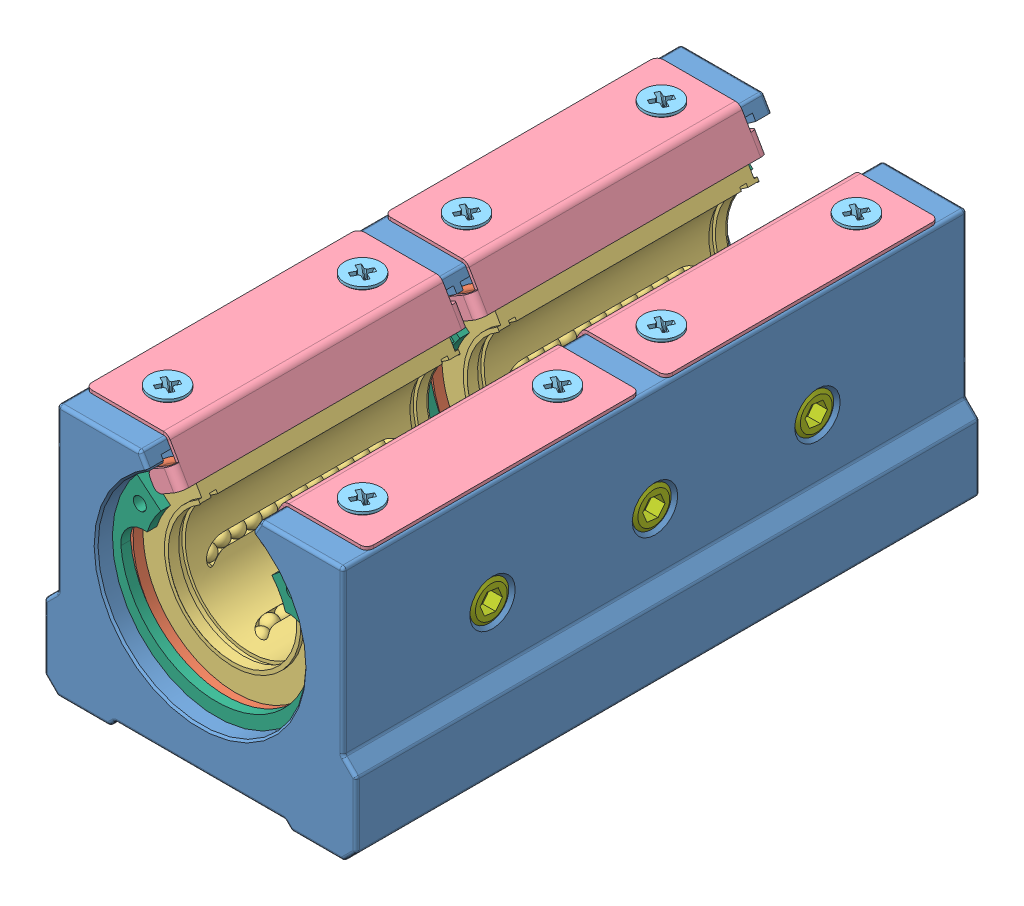
SolidWorks assembly SME20L, configuration Default. Lengths in mm.
Overall size (48 42.63 96.13).
28 component instances, 7 part files, 15 mates.
Components (placement in the parent):
- SME20L-1-1: SME20L-1 [Default] at (-5.7284 29.1482 -16.78) size (48 39.1 96.13)
- LM20OP-2: LM20OP [Default] at (-3.2118 9.9406 8.4417) size (39.07 39.07 42.07)
  - LM20OP-1-2: LM20OP-1 [Default] at (-2.5166 3.2076 -21.2217) size (32 29.9 42.07)
  - LM20OP-2-2: LM20OP-2 [Default] at (4.6334 15.5917 -0.2217) x (0 0 -1) z (-0.5 -0.866025 0) size (40 28.6 28.6)
- SME20L-2-3: SME20L-2 [Default] at (6.4345 29.1482 5.6825) x (1 0 0) z (0 0 -1) size (15.92 7.34 44.47)
- SME20L-2-4: SME20L-2 [Default] at (-17.8913 29.1482 10.7574) x (-1 0 0) z (0 0 1) size (15.92 7.34 44.47)
- countersunk flat head cross recess screw_iso-2: countersunk flat head cross recess screw_iso [ISO 7046-1 - M3 x 4 - Z --- 4N] at (9.2716 30.1892 -6.78) x (0 -1 0) z (-0.452249 0 0.891892) size (4 5.5 5.5)
- countersunk flat head cross recess screw_iso-3: countersunk flat head cross recess screw_iso [ISO 7046-1 - M3 x 4 - Z --- 4N] at (9.2716 30.1892 23.22) x (0 -1 0) z (-0.452249 0 0.891892) size (4 5.5 5.5)
- countersunk flat head cross recess screw_iso-4: countersunk flat head cross recess screw_iso [ISO 7046-1 - M3 x 4 - Z --- 4N] at (-20.7284 30.1892 -6.78) x (0 -1 0) z (-0.452249 0 0.891892) size (4 5.5 5.5)
- countersunk flat head cross recess screw_iso-5: countersunk flat head cross recess screw_iso [ISO 7046-1 - M3 x 4 - Z --- 4N] at (-20.7284 30.1892 23.22) x (0 -1 0) z (-0.452249 0 0.891892) size (4 5.5 5.5)
- SME20L-3-1: SME20L-3 [Default] at (-5.7284 13.1482 29.22) x (-1 0 0) z (0 0 1) size (34 27.93 1.5)
- SME20L-3-2: SME20L-3 [Default] at (-5.7284 13.1482 -14.28) x (-0.999848 0.017452 0) z (0 0 1) size (34 27.93 1.5)
- socket set screw flat point_din-1: socket set screw flat point_din [DIN 913 - M4 x 4-N] at (-5.7284 -8.077 31.22) x (0 1 0) z (0 0 1) size (4 4 4)
- socket set screw flat point_din-2: socket set screw flat point_din [DIN 913 - M6 x 6-N] at (16.0917 13.1482 31.22) x (-1 0 0) z (0 -0.924225 -0.381849) size (6 6 6)
- SME20L-2-5: SME20L-2 [Default] at (-17.8913 29.1482 56.7574) x (-1 0 0) z (0 0 1) size (15.92 7.34 44.47)
- SME20L-2-6: SME20L-2 [Default] at (6.4345 29.1482 51.6825) x (1 0 0) z (0 0 -1) size (15.92 7.34 44.47)
- countersunk flat head cross recess screw_iso-6: countersunk flat head cross recess screw_iso [ISO 7046-1 - M3 x 4 - Z --- 4N] at (9.2716 30.1892 39.22) x (0 -1 0) z (-0.452249 0 0.891892) size (4 5.5 5.5)
- countersunk flat head cross recess screw_iso-7: countersunk flat head cross recess screw_iso [ISO 7046-1 - M3 x 4 - Z --- 4N] at (9.2716 30.1892 69.22) x (0 -1 0) z (-0.452249 0 0.891892) size (4 5.5 5.5)
- countersunk flat head cross recess screw_iso-8: countersunk flat head cross recess screw_iso [ISO 7046-1 - M3 x 4 - Z --- 4N] at (-20.7284 30.1892 39.22) x (0 -1 0) z (-0.452249 0 0.891892) size (4 5.5 5.5)
- countersunk flat head cross recess screw_iso-9: countersunk flat head cross recess screw_iso [ISO 7046-1 - M3 x 4 - Z --- 4N] at (-20.7284 30.1892 69.22) x (0 -1 0) z (-0.452249 0 0.891892) size (4 5.5 5.5)
- LM20OP-3: LM20OP [Default] at (-3.2118 9.9406 54.4417) size (39.07 39.07 42.07)
  - LM20OP-1-2: LM20OP-1 [Default] at (-2.5166 3.2076 -21.2217) size (32 29.9 42.07)
  - LM20OP-2-2: LM20OP-2 [Default] at (4.6334 15.5917 -0.2217) x (0 0 -1) z (-0.5 -0.866025 0) size (40 28.6 28.6)
- SME20L-3-3: SME20L-3 [Default] at (-5.7284 13.1482 31.72) x (-0.999848 0.017452 0) z (0 0 1) size (34 27.93 1.5)
- SME20L-3-4: SME20L-3 [Default] at (-5.7284 13.1482 75.22) x (-1 0 0) z (0 0 1) size (34 27.93 1.5)
- socket set screw flat point_din-3: socket set screw flat point_din [DIN 913 - M6 x 6-N] at (16.0917 13.1482 56.22) x (-1 0 0) z (0 -0.924225 -0.381849) size (6 6 6)
- socket set screw flat point_din-4: socket set screw flat point_din [DIN 913 - M6 x 6-N] at (16.0917 13.1482 6.22) x (-1 0 0) z (0 -0.924225 -0.381849) size (6 6 6)
- socket set screw flat point_din-5: socket set screw flat point_din [DIN 913 - M6 x 6-N] at (16.0917 13.1482 31.22) x (-1 0 0) z (0 -0.924225 -0.381849) size (6 6 6)
Mates (geometry in assembly coordinates):
- Concentric2: concentric aligned: cylinder of SME20L-1-1 through (-5.7284 13.1482 79.22) axis (0 0 -1) radius 16; cylinder of LM20OP-2/LM20OP-1-2 through (-5.7284 13.1482 29.22) axis (0 0 -1) radius 16
- Coincident7: coincident anti-aligned: plane of SME20L-1-1 through (3.5092 29.1482 79.22) normal (0 1 0); plane of SME20L-2-3 through (15.9345 29.1482 -12.78) normal (0 -1 0)
- Coincident8: coincident anti-aligned: plane of SME20L-1-1 through (2.2716 27.0046 79.22) normal (-0.866025 0.5 0); plane of SME20L-2-3 through (9.944 40.2937 -12.78) normal (0.866025 -0.5 0)
- Coincident9: coincident aligned: plane of LM20OP-2/LM20OP-1-2 through (-5.7284 13.1482 29.22) normal (0 0 1); plane of SME20L-2-3 through (-0.0655 29.6482 29.22) normal (0 0 1)
- Coincident10: coincident anti-aligned: plane of SME20L-1-1 through (-14.966 29.1482 79.22) normal (0 1 0); plane of SME20L-2-4 through (-27.3913 29.1482 29.22) normal (0 -1 0)
- Coincident11: coincident anti-aligned: plane of SME20L-1-1 through (-13.7284 27.0046 79.22) normal (0.866025 0.5 0); plane of SME20L-2-4 through (-21.4009 40.2937 29.22) normal (-0.866025 -0.5 0)
- Coincident12: coincident aligned: plane of LM20OP-2/LM20OP-1-2 through (-5.7284 13.1482 29.22) normal (0 0 1); plane of SME20L-2-4 through (-11.3913 29.6482 29.22) normal (0 0 1)
- Coincident13: coincident anti-aligned: plane of SME20L-1-1 through (-5.7284 -2.8518 30.72) normal (0 0 -1); plane of SME20L-3-1 through (-5.7284 13.1482 30.72) normal (0 0 1)
- Concentric6: concentric anti-aligned: cylinder of SME20L-1-1 through (-5.7284 13.1482 33.22) axis (0 0 1) radius 17; cylinder of SME20L-3-1 through (-5.7284 13.1482 30.72) axis (0 0 -1) radius 17
- Coincident15: coincident anti-aligned: plane of SME20L-1-1 through (-5.7284 -2.8518 -14.28) normal (0 0 1); plane of SME20L-3-2 through (-5.7284 13.1482 -14.28) normal (0 0 -1)
- Concentric7: concentric anti-aligned: cylinder of SME20L-1-1 through (-5.7284 13.1482 33.22) axis (0 0 1) radius 17; cylinder of SME20L-3-2 through (-5.7284 13.1482 -12.78) axis (0 0 -1) radius 17
- Concentric8: concentric aligned: cylinder of SME20L-1-1 through (-5.7284 29.1492 31.22) axis (0 -1 0) radius 2; cylinder of socket set screw flat point_din-1 through (-5.7284 -20.777 31.22) axis (0 -1 0) radius 2
- Coincident16: coincident aligned: circle of SME20L-1-1; circle of socket set screw flat point_din-1
- Concentric9: concentric aligned: cylinder of SME20L-1-1 through (-29.7294 13.1482 31.22) axis (1 0 0) radius 3; cylinder of socket set screw flat point_din-2 through (28.7917 13.1482 31.22) axis (1 0 0) radius 3
- Coincident17: coincident aligned: circle of SME20L-1-1; circle of socket set screw flat point_din-2
